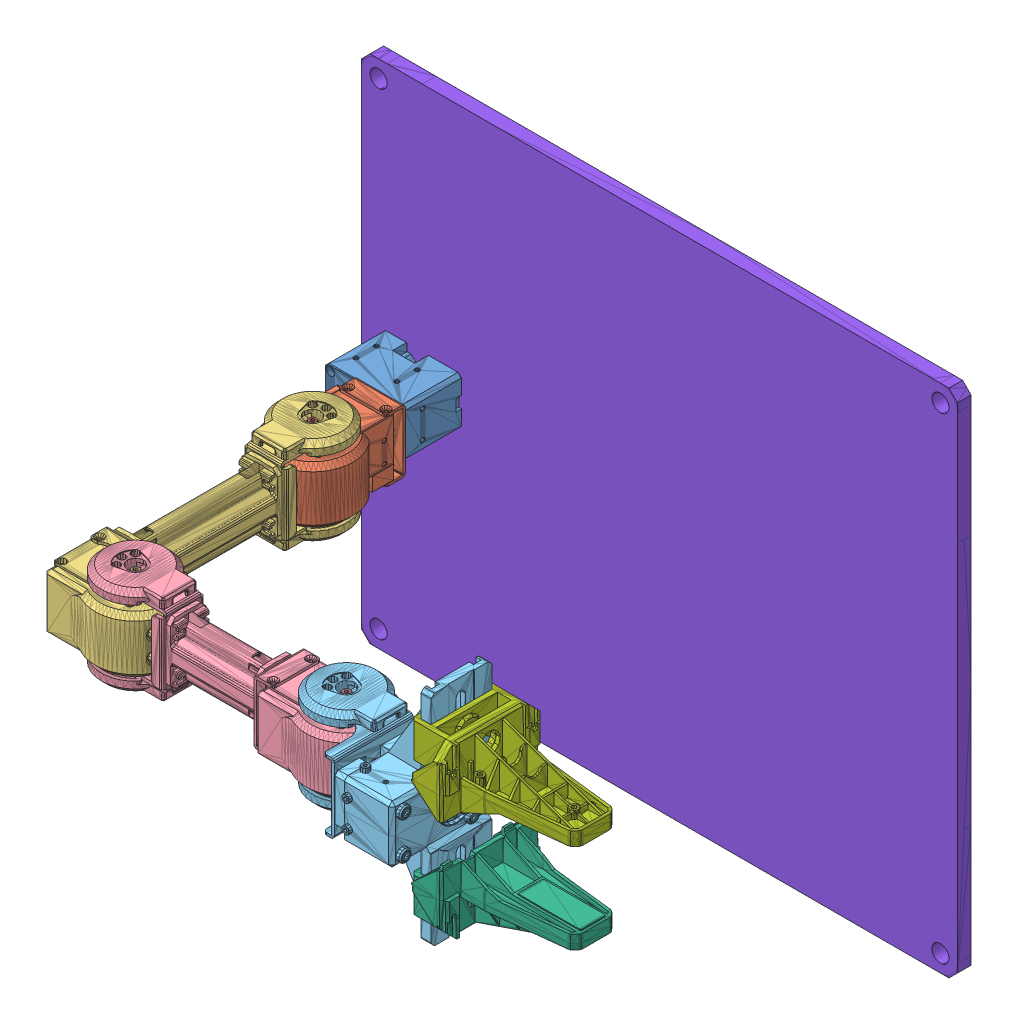
SolidWorks assembly OpenMANIPULATOR-X, configuration Default. Lengths in mm.
Overall size (350 300 252.25).
8 component instances, 8 part files, 21 mates.
Components (placement in the parent):
- chain_link1-1: chain_link1 [Default] at origin size (46.5 28.5 40.4)
- chain_link2-1: chain_link2 [Default] at (12 0.0001 36) size (47 42.4 63.83)
- chain_link3-1: chain_link3 [Default] at (12 0.0001 76.5) size (67.35 52 171.49)
- chain_link4-1: chain_link4 [Default] at (35.9999 0.0001 204.5) size (167.32 52.6 47)
- chain_link5-1: chain_link5 [Default] at (159.9998 0.0001 204.5001) size (88.39 128.6 62.75)
- chain_link_grip_r-1: chain_link_grip_r [Default] at (241.6998 -21.6999 204.5001) size (88.1 39.75 58)
- chain_link_grip_l-1: chain_link_grip_l [Default] at (241.6998 21.7001 204.5001) size (88.1 39.75 58)
- OpenMANIPULATOR_Plate-1: OpenMANIPULATOR_Plate [Default] at (12.0462 -0.2561 0) size (350 300 8)
Mates (geometry in assembly coordinates):
- Concentric1: concentric anti-aligned: circle of chain_link1-1; circle of chain_link2-1
- Coincident1: coincident anti-aligned: plane of chain_link1-1 through (0 0 36) normal (0 0 1); plane of chain_link2-1 through (12 0.0001 36) normal (0 0 -1)
- Parallel1: parallel aligned: plane of chain_link1-1 through (23.25 0 0) normal (1 0 0); plane of chain_link2-1 through (26.0001 0.0001 36) normal (1 0 0)
- Concentric2: concentric aligned: circle of chain_link2-1; circle of chain_link3-1
- Coincident3: coincident anti-aligned: plane of chain_link2-1 through (12 -18.9999 36) normal (0 -1 0); plane of chain_link3-1 through (12 -18.9999 76.5) normal (0 1 0)
- Parallel3: parallel anti-aligned: plane of chain_link1-1 through (0 0 34) normal (0 0 1); plane of chain_link3-1 through (12 0.0001 185) normal (0 0 -1)
- Concentric3: concentric aligned: circle of chain_link3-1; circle of chain_link4-1
- Perpendicular1: perpendicular: plane of chain_link3-1 through (18.5 -6.4999 76.5) normal (0.707107 -0.707107 0); plane of chain_link4-1 through (35.9999 0.0001 215) normal (0 0 1)
- Coincident7: coincident anti-aligned: plane of chain_link3-1 through (12 -18.9999 76.5) normal (0 -1 0); plane of chain_link4-1 through (35.9999 -18.9999 204.5) normal (0 1 0)
- Concentric4: concentric aligned: circle of chain_link4-1; circle of chain_link5-1
- Coincident8: coincident anti-aligned: plane of chain_link4-1 through (35.9999 -18.9999 204.5) normal (0 -1 0); plane of chain_link5-1 through (159.9998 -18.9999 204.5001) normal (0 1 0)
- Parallel4: parallel aligned: plane of chain_link4-1 through (35.9999 0.0001 215) normal (0 0 1); plane of chain_link5-1 through (159.9998 0.0001 242.3001) normal (0 0 1)
- Distance2: distance = 0.1 mm anti-aligned: plane of chain_link5-1 through (221.4998 0.0001 204.5001) normal (-1 0 0); plane of chain_link_grip_r-1 through (221.3998 -21.6999 204.5001) normal (1 0 0)
- Distance1: distance = 0.1 mm anti-aligned: plane of chain_link5-1 through (159.9998 0.0001 190.0001) normal (0 0 1); plane of chain_link_grip_r-1 through (241.6998 -21.6999 190.1001) normal (0 0 -1)
- Distance3: distance = 15 mm aligned: plane of chain_link5-1 through (159.9998 -64.2999 204.5001) normal (0 -1 0); plane of chain_link_grip_r-1 through (241.6998 -49.2999 204.5001) normal (0 -1 0)
- Coincident16: coincident: plane of chain_link_grip_r-1 through (221.3998 -21.6999 204.5001) normal (1 0 0); plane of chain_link_grip_l-1 through (221.3998 21.7001 204.5001) normal (1 0 0)
- Coincident17: coincident: plane of chain_link_grip_r-1 through (241.6998 -21.6999 186.5001) normal (0 0 1); plane of chain_link_grip_l-1 through (241.6998 21.7001 186.5001) normal (0 0 1)
- Distance4: distance = 15 mm aligned: plane of chain_link_grip_l-1 through (241.6998 49.3001 204.5001) normal (0 1 0); plane of chain_link5-1 through (159.9998 64.3001 204.5001) normal (0 1 0)
- Concentric5: concentric: circle of chain_link1-1; circle of OpenMANIPULATOR_Plate-1
- Coincident19: coincident: plane of chain_link1-1 through (0 0 0) normal (0 0 -1); plane of OpenMANIPULATOR_Plate-1 through (12.0462 -0.2561 0) normal (0 0 1)
- Parallel5: parallel aligned: plane of chain_link1-1 through (0 14.25 0) normal (0 1 0); plane of OpenMANIPULATOR_Plate-1 through (-35.75 150 -8) normal (0 1 0)
